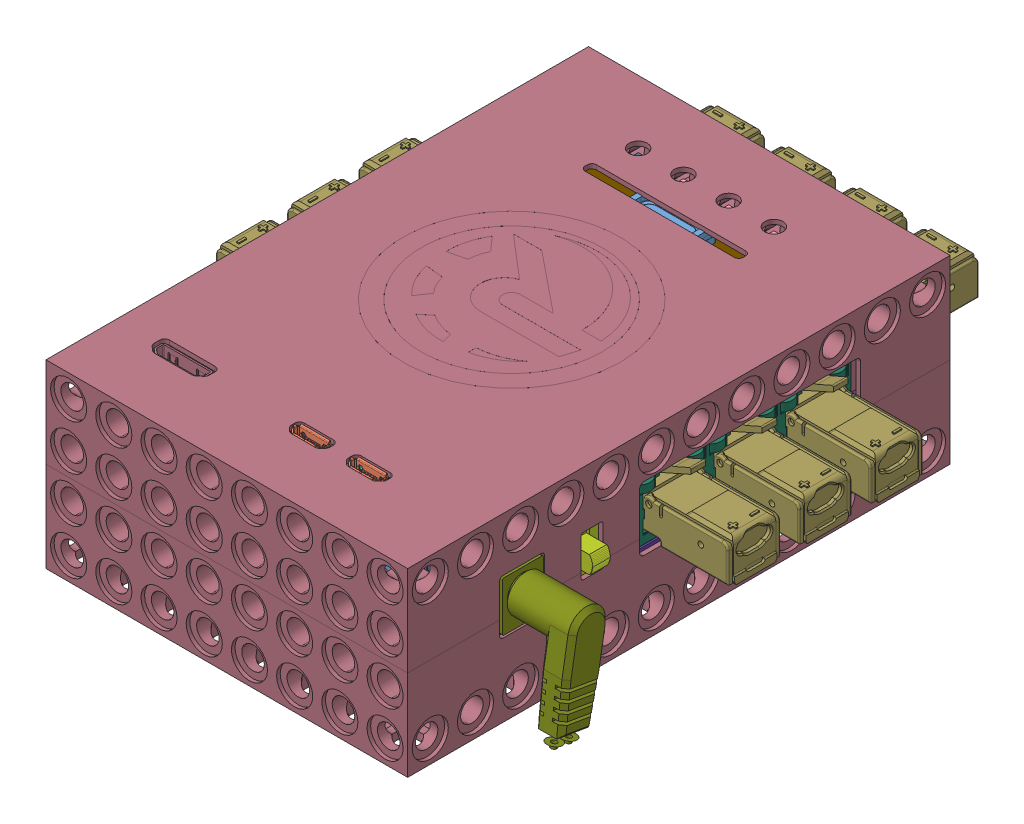
SolidWorks assembly PCBA_estimation_20190215, configuration Default. Lengths in mm. (continued)
Components (placement in the parent): (continued)
- RRRC_carrier_board-1: RRRC_carrier_board [Default] at (75.1836 8.28 47.3515) x (0 0 -1) z (0 1 0) size (102.74 81.4 21.81) (continued)
  - D1_CARRIER_3-1: D1_CARRIER_3 [Default] at origin size (1.05 0.65 0.44)
    - SOD-923_3-1: SOD-923_3 [Default] at (75.25 23.35 0) x (1 0 0) z (0 -1 0) size (1.05 0.44 0.65)
  - CON8_CARRIER_3-1: CON8_CARRIER_3 [Default] at origin size (17.2 66.95 18.85)
    - M-RJHSE-X38X-04-REVG1_3-1: M-RJHSE-X38X-04-REVG1_3 [Default] at (102.2431 7.1312 0.09) x (0 1 0) z (1 0 0) size (66.95 18.85 17.2)
  - CON7_CARRIER_3-1: CON7_CARRIER_3 [Default] at origin size (12.84 51.3 8.23)
    - Sullins_PPTC202LJBN-RC_3-1: Sullins_PPTC202LJBN-RC_3 [Default] at (8.4599 17.8499 -1.61) x (0 1 0) z (0 0 1) size (51.3 12.84 8.23)
  - CON6_CARRIER_3-1: CON6_CARRIER_3 [Default] at origin size (6.35 2.14 6.3)
    - SULLINS_GRPB051VWVN-RC_3-1: SULLINS_GRPB051VWVN-RC_3 [Default] at (-23.9866 70.2239 0) x (-1 0 0) z (0 1 0) size (6.35 6.3 2.14)
  - CON5_CARRIER_3-1: CON5_CARRIER_3 [Default] at origin size (3.02 8.01 9.01)
    - Molex_1051330001_3-1: Molex_1051330001_3 [Default] at (15.95 31.8001 2.7) x (0 1 0) z (0 0 -1) size (8.01 3.02 9.01)
  - CON4_CARRIER_3-1: CON4_CARRIER_3 [Default] at origin size (9 14.5 14.5)
    - CUI_INC_PJ-037A_3-1: CUI_INC_PJ-037A_3 [Default] at (9.6999 -1.4998 0) x (1 0 0) z (0 -1 0) size (9 14.5 14.5)
  - CON3_CARRIER_3-1: CON3_CARRIER_3 [Default] at origin size (51.17 16.61 18.92)
    - FCI_RJHSE538103-REVT1_3-1: FCI_RJHSE538103-REVT1_3 [Default] at (44.3006 76.8304 0.65) x (-1 0 0) z (0 1 0) size (51.17 18.92 16.61)
  - C58_CARRIER_3-1: C58_CARRIER_3 [Default] at origin size (1 0.5 0.5)
    - C_0402_3-1: C_0402_3 [Default] at (69.9 48.5 0) x (-1 0 0) z (0 0 1) size (1 0.5 0.5)
  - C38_CARRIER_3-1: C38_CARRIER_3 [Default] at origin size (0.5 1 0.5)
    - C_0402_3-1: C_0402_3 [Default] at (75.175 29.6 0) x (0 1 0) z (0 0 1) size (1 0.5 0.5)
  - C116_CARRIER_3-1: C116_CARRIER_3 [Default] at origin size (1 0.5 0.5)
    - C_0402_3-1: C_0402_3 [Default] at (71.9 53 0) x (1 0 0) z (0 0 1) size (1 0.5 0.5)
  - C115_CARRIER_3-1: C115_CARRIER_3 [Default] at origin size (1 0.5 0.5)
    - C_0402_3-1: C_0402_3 [Default] at (69.9 53 0) x (-1 0 0) z (0 0 1) size (1 0.5 0.5)
  - C114_CARRIER_3-1: C114_CARRIER_3 [Default] at origin size (0.5 1 0.5)
    - C_0402_3-1: C_0402_3 [Default] at (93.75 3 0) x (0 1 0) z (0 0 1) size (1 0.5 0.5)
  - C113_CARRIER_3-1: C113_CARRIER_3 [Default] at origin size (1 0.5 0.5)
    - C_0402_3-1: C_0402_3 [Default] at (71.95 39.35 0) x (1 0 0) z (0 0 1) size (1 0.5 0.5)
  - C109_CARRIER_3-1: C109_CARRIER_3 [Default] at origin size (1 0.5 0.5)
    - C_0402_3-1: C_0402_3 [Default] at (69.95 39.35 0) x (-1 0 0) z (0 0 1) size (1 0.5 0.5)
  - C108_CARRIER_3-1: C108_CARRIER_3 [Default] at origin size (1 0.5 0.5)
    - C_0402_3-1: C_0402_3 [Default] at (77.85 19.25 0) x (-1 0 0) z (0 0 1) size (1 0.5 0.5)
  - C107_CARRIER_3-1: C107_CARRIER_3 [Default] at origin size (1.6 3.2 1.6)
    - C_1206_3-1: C_1206_3 [Default] at (78.15 23.9 0) x (0 -1 0) z (0 0 1) size (3.2 1.6 1.6)
  - C106_CARRIER_3-1: C106_CARRIER_3 [Default] at origin size (3.2 1.6 1.6)
    - C_1206_3-1: C_1206_3 [Default] at (78.95 27.6 0) x (1 0 0) z (0 0 1) size (3.2 1.6 1.6)
  - C104_CARRIER_3-1: C104_CARRIER_3 [Default] at origin size (1 0.5 0.5)
    - C_0402_3-1: C_0402_3 [Default] at (71.9 43.825 0) x (1 0 0) z (0 0 1) size (1 0.5 0.5)
  - C98_CARRIER_3-1: C98_CARRIER_3 [Default] at origin size (1 0.5 0.5)
    - C_0402_3-1: C_0402_3 [Default] at (69.9 43.825 0) x (-1 0 0) z (0 0 1) size (1 0.5 0.5)
  - C97_CARRIER_3-1: C97_CARRIER_3 [Default] at origin size (1.6 3.2 1.6)
    - C_1206_3-1: C_1206_3 [Default] at (30.9 62.1 0) x (0 -1 0) z (0 0 1) size (3.2 1.6 1.6)
  - C96_CARRIER_3-1: C96_CARRIER_3 [Default] at origin size (1 0.5 0.5)
    - C_0402_3-1: C_0402_3 [Default] at (71.9 48.5 0) x (1 0 0) z (0 0 1) size (1 0.5 0.5)
  - C95_CARRIER_3-1: C95_CARRIER_3 [Default] at origin size (1 0.5 0.5)
    - C_0402_3-1: C_0402_3 [Default] at (16.6 19.725 0) x (1 0 0) z (0 0 1) size (1 0.5 0.5)
  - C94_CARRIER_3-1: C94_CARRIER_3 [Default] at origin size (1.6 3.2 1.6)
    - C_1206_3-1: C_1206_3 [Default] at (32.75 12.9 0) x (0 1 0) z (0 0 1) size (3.2 1.6 1.6)
  - C93_CARRIER_3-1: C93_CARRIER_3 [Default] at origin size (1.6 3.2 1.6)
    - C_1206_3-1: C_1206_3 [Default] at (17.05 12.9 0) x (0 1 0) z (0 0 1) size (3.2 1.6 1.6)
  - C92_CARRIER_3-1: C92_CARRIER_3 [Default] at origin size (1.6 3.2 1.6)
    - C_1206_3-1: C_1206_3 [Default] at (3.4 10.65 0) x (0 1 0) z (0 0 1) size (3.2 1.6 1.6)
  - C91_CARRIER_3-1: C91_CARRIER_3 [Default] at origin size (0.5 1 0.5)
    - C_0402_3-1: C_0402_3 [Default] at (88.95 74.5 0) x (0 -1 0) z (0 0 1) size (1 0.5 0.5)
  - C89_CARRIER_3-1: C89_CARRIER_3 [Default] at origin size (1.6 3.2 1.6)
    - C_1206_3-1: C_1206_3 [Default] at (20.075 27.05 0) x (0 -1 0) z (0 0 1) size (3.2 1.6 1.6)
  - C88_CARRIER_3-1: C88_CARRIER_3 [Default] at origin size (1 0.5 0.5)
    - C_0402_3-1: C_0402_3 [Default] at (66.9 56.6 0) x (1 0 0) z (0 0 1) size (1 0.5 0.5)
  - C87_CARRIER_3-1: C87_CARRIER_3 [Default] at origin size (1 0.5 0.5)
    - C_0402_3-1: C_0402_3 [Default] at (62.45 57.7 0) x (-1 0 0) z (0 0 1) size (1 0.5 0.5)
  - C85_CARRIER_3-1: C85_CARRIER_3 [Default] at origin size (1.2 2 1.2)
    - C_0805_3-1: C_0805_3 [Default] at (64.45 51.95 0.1) x (0 -1 0) z (0 0 1) size (2 1.2 1.2)
  - C83_CARRIER_3-1: C83_CARRIER_3 [Default] at origin size (1 0.5 0.5)
    - C_0402_3-1: C_0402_3 [Default] at (69.25 55.05 0) x (1 0 0) z (0 0 1) size (1 0.5 0.5)
  - C80_CARRIER_3-1: C80_CARRIER_3 [Default] at origin size (0.5 1 0.5)
    - C_0402_3-1: C_0402_3 [Default] at (79.875 22.925 0) x (0 -1 0) z (0 0 1) size (1 0.5 0.5)
  - C78_CARRIER_3-1: C78_CARRIER_3 [Default] at origin size (0.5 1 0.5)
    - C_0402_3-1: C_0402_3 [Default] at (79.85 25.425 0) x (0 1 0) z (0 0 1) size (1 0.5 0.5)
  - C69_CARRIER_3-1: C69_CARRIER_3 [Default] at origin size (1 0.5 0.5)
    - C_0402_3-1: C_0402_3 [Default] at (32.75 28.7 0) x (-1 0 0) z (0 0 1) size (1 0.5 0.5)
  - C68_CARRIER_3-1: C68_CARRIER_3 [Default] at origin size (1 0.5 0.5)
    - C_0402_3-1: C_0402_3 [Default] at (32.75 32.5 0) x (-1 0 0) z (0 0 1) size (1 0.5 0.5)
  - C67_CARRIER_3-1: C67_CARRIER_3 [Default] at origin size (0.5 1 0.5)
    - C_0402_3-1: C_0402_3 [Default] at (18.4 26.25 0) x (0 1 0) z (0 0 1) size (1 0.5 0.5)
  - C66_CARRIER_3-1: C66_CARRIER_3 [Default] at origin size (0.5 1 0.5)
    - C_0402_3-1: C_0402_3 [Default] at (19.475 30.6 0) x (0 1 0) z (0 0 1) size (1 0.5 0.5)
  - C65_CARRIER_3-1: C65_CARRIER_3 [Default] at origin size (1.6 3.2 1.6)
    - C_1206_3-1: C_1206_3 [Default] at (7.15 22.3 0) x (0 -1 0) z (0 0 1) size (3.2 1.6 1.6)
  - C64_CARRIER_3-1: C64_CARRIER_3 [Default] at origin size (0.5 1 0.5)
    - C_0402_3-1: C_0402_3 [Default] at (22.5 30.6 0) x (0 1 0) z (0 0 1) size (1 0.5 0.5)
  - C62_CARRIER_3-1: C62_CARRIER_3 [Default] at origin size (1 0.5 0.5)
    - C_0402_3-1: C_0402_3 [Default] at (33.025 62.8 0) x (-1 0 0) z (0 0 1) size (1 0.5 0.5)
  - C61_CARRIER_3-1: C61_CARRIER_3 [Default] at origin size (0.5 1 0.5)
    - C_0402_3-1: C_0402_3 [Default] at (7.325 64.75 0) x (0 -1 0) z (0 0 1) size (1 0.5 0.5)
  - C60_CARRIER_3-1: C60_CARRIER_3 [Default] at origin size (0.5 1 0.5)
    - C_0402_3-1: C_0402_3 [Default] at (7.325 66.75 0) x (0 1 0) z (0 0 1) size (1 0.5 0.5)
  - C59_CARRIER_3-1: C59_CARRIER_3 [Default] at origin size (2 1.2 1.2)
    - C_0805_3-1: C_0805_3 [Default] at (4.25 36.05 0.1) x (1 0 0) z (0 0 1) size (2 1.2 1.2)
  - C57_CARRIER_3-1: C57_CARRIER_3 [Default] at origin size (0.5 1 0.5)
    - C_0402_3-1: C_0402_3 [Default] at (14.95 21.275 0) x (0 -1 0) z (0 0 1) size (1 0.5 0.5)
  - C56_CARRIER_3-1: C56_CARRIER_3 [Default] at origin size (0.81 1.6 0.81)
    - C_0603_3-1: C_0603_3 [Default] at (6.5 30 0) x (0 -1 0) z (0 0 1) size (1.6 0.81 0.81)
  - C55_CARRIER_3-1: C55_CARRIER_3 [Default] at origin size (0.5 1 0.5)
    - C_0402_3-1: C_0402_3 [Default] at (1.2 51.75 0) x (0 1 0) z (0 0 1) size (1 0.5 0.5)
  - C54_CARRIER_3-1: C54_CARRIER_3 [Default] at origin size (1.6 3.2 1.6)
    - C_1206_3-1: C_1206_3 [Default] at (62.45 52.5 0) x (0 -1 0) z (0 0 1) size (3.2 1.6 1.6)
  - C52_CARRIER_3-1: C52_CARRIER_3 [Default] at origin size (1.6 3.2 1.6)
    - C_1206_3-1: C_1206_3 [Default] at (50.3 52.15 0) x (0 1 0) z (0 0 1) size (3.2 1.6 1.6)
  - C50_CARRIER_3-1: C50_CARRIER_3 [Default] at origin size (1.6 3.2 1.6)
    - C_1206_3-1: C_1206_3 [Default] at (42.1 51.85 0) x (0 1 0) z (0 0 1) size (3.2 1.6 1.6)
  - C48_CARRIER_3-1: C48_CARRIER_3 [Default] at origin size (1.6 3.2 1.6)
    - C_1206_3-1: C_1206_3 [Default] at (37.375 25.625 0) x (0 1 0) z (0 0 1) size (3.2 1.6 1.6)
  - C47_CARRIER_3-1: C47_CARRIER_3 [Default] at origin size (3.2 1.6 1.6)
    - C_1206_3-1: C_1206_3 [Default] at (34.325 18.15 0) x (-1 0 0) z (0 0 1) size (3.2 1.6 1.6)
  - C44_CARRIER_3-1: C44_CARRIER_3 [Default] at origin size (2 1.2 1.2)
    - C_0805_3-1: C_0805_3 [Default] at (3.9 60.9 0.1) x (1 0 0) z (0 0 1) size (2 1.2 1.2)
  - C43_CARRIER_3-1: C43_CARRIER_3 [Default] at origin size (0.81 1.6 0.81)
    - C_0603_3-1: C_0603_3 [Default] at (6.525 54.375 0) x (0 1 0) z (0 0 1) size (1.6 0.81 0.81)
  - C40_CARRIER_3-1: C40_CARRIER_3 [Default] at origin size (0.5 1 0.5)
    - C_0402_3-1: C_0402_3 [Default] at (5.05 23.25 0) x (0 1 0) z (0 0 1) size (1 0.5 0.5)
  - C45_CARRIER_3-1: C45_CARRIER_3 [Default] at origin size (0.5 1 0.5)
    - C_0402_3-1: C_0402_3 [Default] at (47.15 29.6 0) x (0 1 0) z (0 0 1) size (1 0.5 0.5)
  - C41_CARRIER_3-1: C41_CARRIER_3 [Default] at origin size (0.5 1 0.5)
    - C_0402_3-1: C_0402_3 [Default] at (60.15 29.6 0) x (0 1 0) z (0 0 1) size (1 0.5 0.5)
  - C26_CARRIER_3-1: C26_CARRIER_3 [Default] at origin size (3.2 1.6 1.6)
    - C_1206_3-1: C_1206_3 [Default] at (61.15 37.95 0) x (1 0 0) z (0 0 1) size (3.2 1.6 1.6)
  - C22_CARRIER_3-1: C22_CARRIER_3 [Default] at origin size (1.6 3.2 1.6)
    - C_1206_3-1: C_1206_3 [Default] at (70.725 33.025 0) x (0 1 0) z (0 0 1) size (3.2 1.6 1.6)
  - C20_CARRIER_3-1: C20_CARRIER_3 [Default] at origin size (1 0.5 0.5)
    - C_0402_3-1: C_0402_3 [Default] at (65.175 35.8 0) x (-1 0 0) z (0 0 1) size (1 0.5 0.5)
  - C18_CARRIER_3-1: C18_CARRIER_3 [Default] at origin size (0.5 1 0.5)
    - C_0402_3-1: C_0402_3 [Default] at (72.35 34.25 0) x (0 1 0) z (0 0 1) size (1 0.5 0.5)
  - C17_CARRIER_3-1: C17_CARRIER_3 [Default] at origin size (1 0.5 0.5)
    - C_0402_3-1: C_0402_3 [Default] at (69.325 19.575 0) x (-1 0 0) z (0 0 1) size (1 0.5 0.5)
  - C16_CARRIER_3-1: C16_CARRIER_3 [Default] at origin size (1 0.5 0.5)
    - C_0402_3-1: C_0402_3 [Default] at (73.375 19.575 0) x (-1 0 0) z (0 0 1) size (1 0.5 0.5)
  - C15_CARRIER_3-1: C15_CARRIER_3 [Default] at origin size (1 0.5 0.5)
    - C_0402_3-1: C_0402_3 [Default] at (70.85 22.55 0) x (1 0 0) z (0 0 1) size (1 0.5 0.5)
  - C14_CARRIER_3-1: C14_CARRIER_3 [Default] at origin size (2 1.2 1.2)
    - C_0805_3-1: C_0805_3 [Default] at (75.2 21.85 0.1) x (1 0 0) z (0 0 1) size (2 1.2 1.2)
  - C13_CARRIER_3-1: C13_CARRIER_3 [Default] at origin size (0.5 1 0.5)
    - C_0402_3-1: C_0402_3 [Default] at (15.55 44.05 0) x (0 -1 0) z (0 0 1) size (1 0.5 0.5)
  - C12_CARRIER_3-1: C12_CARRIER_3 [Default] at origin size (0.5 1 0.5)
    - C_0402_3-1: C_0402_3 [Default] at (15.35 48.85 0) x (0 -1 0) z (0 0 1) size (1 0.5 0.5)
  - C11_CARRIER_3-1: C11_CARRIER_3 [Default] at origin size (0.5 1 0.5)
    - C_0402_3-1: C_0402_3 [Default] at (35.3 54.025 0) x (0 1 0) z (0 0 1) size (1 0.5 0.5)
  - C10_CARRIER_3-1: C10_CARRIER_3 [Default] at origin size (1 0.5 0.5)
    - C_0402_3-1: C_0402_3 [Default] at (23.4 57.76 0) x (-1 0 0) z (0 0 1) size (1 0.5 0.5)
  - C9_CARRIER_3-1: C9_CARRIER_3 [Default] at origin size (1 0.5 0.5)
    - C_0402_3-1: C_0402_3 [Default] at (27 57.75 0) x (-1 0 0) z (0 0 1) size (1 0.5 0.5)
  - C8_CARRIER_3-1: C8_CARRIER_3 [Default] at origin size (1 0.5 0.5)
    - C_0402_3-1: C_0402_3 [Default] at (29.55 57.76 0) size (1 0.5 0.5)
  - C7_CARRIER_3-1: C7_CARRIER_3 [Default] at origin size (1 0.5 0.5)
    - C_0402_3-1: C_0402_3 [Default] at (22.1 38.15 0) x (1 0 0) z (0 0 1) size (1 0.5 0.5)
  - C6_CARRIER_3-1: C6_CARRIER_3 [Default] at origin size (1 0.5 0.5)
    - C_0402_3-1: C_0402_3 [Default] at (26.5 38.05 0) x (-1 0 0) z (0 0 1) size (1 0.5 0.5)
  - C5_CARRIER_3-1: C5_CARRIER_3 [Default] at origin size (1 0.5 0.5)
    - C_0402_3-1: C_0402_3 [Default] at (26.5 37.05 0) x (-1 0 0) z (0 0 1) size (1 0.5 0.5)
  - C4_CARRIER_3-1: C4_CARRIER_3 [Default] at origin size (0.5 1 0.5)
    - C_0402_3-1: C_0402_3 [Default] at (35.25 51.4 0) x (0 1 0) z (0 0 1) size (1 0.5 0.5)
  - C3_CARRIER_3-1: C3_CARRIER_3 [Default] at origin size (3.2 1.6 1.6)
    - C_1206_3-1: C_1206_3 [Default] at (38.3 51.75 0) x (-1 0 0) z (0 0 1) size (3.2 1.6 1.6)
  - C2_CARRIER_3-1: C2_CARRIER_3 [Default] at origin size (1.6 3.2 1.6)
    - C_1206_3-1: C_1206_3 [Default] at (33.15 59.775 0) x (0 -1 0) z (0 0 1) size (3.2 1.6 1.6)
  - C1_CARRIER_3-1: C1_CARRIER_3 [Default] at origin size (0.5 1 0.5)
    - C_0402_3-1: C_0402_3 [Default] at (22.95 35.55 0) x (0 1 0) z (0 0 1) size (1 0.5 0.5)
- RRRC_LED_board-1: RRRC_LED_board [Default] at (7.6864 26.7896 -45.8485) x (0 0 1) z (0 1 0) size (80 58 5.61)
  - Board_LEDs-1: Board_LEDs [Default] at origin size (80 58 1.6)
    - Open CASCADE STEP translator 6.8 1.1.1_3-1: Open CASCADE STEP translator 6.8 1.1.1_3 [Default] at (0 0 -1.6) size (80 58 1.6)
  - LS2_LEDs-1: LS2_LEDs [Default] at origin size (11 15 4.4)
    - AS01508AO-SC-R-1: AS01508AO-SC-R [Default] at (9.1999 22.6001 2.05) x (0 1 0) z (0 0 -1) size (15 11 4.4)
  - R2_LEDs-1: R2_LEDs [Default] at origin size (0.55 1.15 0.41)
    - R_0402_4-1: R_0402_4 [Default] at (15.225 50.25 0) x (0 -1 0) z (-1 0 0) size (1.15 0.41 0.55)
  - R1_LEDs-1: R1_LEDs [Default] at origin size (0.55 1.15 0.41)
    - R_0402_4-1: R_0402_4 [Default] at (9.325 49.825 0) x (0 -1 0) z (-1 0 0) size (1.15 0.41 0.55)
  - Q1_LEDs-1: Q1_LEDs [Default] at origin size (3 3.05 1.41)
    - SOT95P255X140-3N_4-1: SOT95P255X140-3N_4 [Default] at (12.15 50.275 0) x (-1 0 0) z (0 0 1) size (3 3.05 1.41)
  - LED16_LEDs-1: LED16_LEDs [Default] at origin size (5 5 1.6)
    - 6300770016-1: 6300770016 [Default] at (46 7 0) size (5 5 1.6)
      - Extruded_4-1: Extruded_4 [Default] at origin size (5 5 1.6)
  - LED15_LEDs-1: LED15_LEDs [Default] at origin size (6.83 6.83 1.6)
    - 6300767936-1: 6300767936 [Default] at (57 9.9474 0) size (6.83 6.83 1.6)
      - Extruded_4_2-1: Extruded_4_2 [Default] at origin size (6.83 6.83 1.6)
  - LED14_LEDs-1: LED14_LEDs [Default] at origin size (6.83 6.83 1.6)
    - 6300767056-1: 6300767056 [Default] at (65.0526 18 0) size (6.83 6.83 1.6)
      - Extruded_4_3-1: Extruded_4_3 [Default] at origin size (6.83 6.83 1.6)
  - LED13_LEDs-1: LED13_LEDs [Default] at origin size (5 5 1.6)
    - 6300770016-1-1: 6300770016-1 [Default] at (68 29 0) size (5 5 1.6)
      - Extruded_4-1: Extruded_4 [Default] at origin size (5 5 1.6)
  - LED12_LEDs-1: LED12_LEDs [Default] at origin size (6.83 6.83 1.6)
    - 6300767936-1-1: 6300767936-1 [Default] at (65.0526 40 0) size (6.83 6.83 1.6)
      - Extruded_4_2-1: Extruded_4_2 [Default] at origin size (6.83 6.83 1.6)
  - LED11_LEDs-1: LED11_LEDs [Default] at origin size (6.83 6.83 1.6)
    - 6300767056-1-1: 6300767056-1 [Default] at (57 48.0526 0) size (6.83 6.83 1.6)
      - Extruded_4_3-1: Extruded_4_3 [Default] at origin size (6.83 6.83 1.6)
  - LED10_LEDs-1: LED10_LEDs [Default] at origin size (5 5 1.6)
    - 6300770016-2-1: 6300770016-2 [Default] at (46 51 0) size (5 5 1.6)
      - Extruded_4-1: Extruded_4 [Default] at origin size (5 5 1.6)
  - LED9_LEDs-1: LED9_LEDs [Default] at origin size (6.83 6.83 1.6)
    - 6300765456-1: 6300765456 [Default] at (35 48.0526 0) size (6.83 6.83 1.6)
      - Extruded_4_4-1: Extruded_4_4 [Default] at origin size (6.83 6.83 1.6)
  - LED8_LEDs-1: LED8_LEDs [Default] at origin size (6.83 6.83 1.6)
    - 6300764256-1: 6300764256 [Default] at (26.9474 40 0) size (6.83 6.83 1.6)
      - Extruded_4_5-1: Extruded_4_5 [Default] at origin size (6.83 6.83 1.6)
  - LED7_LEDs-1: LED7_LEDs [Default] at origin size (5 5 1.6)
    - 6300770016-3-1: 6300770016-3 [Default] at (24 29 0) size (5 5 1.6)
      - Extruded_4-1: Extruded_4 [Default] at origin size (5 5 1.6)
  - LED6_LEDs-1: LED6_LEDs [Default] at origin size (6.83 6.83 1.6)
    - 6300767936-2-1: 6300767936-2 [Default] at (26.9474 18 0) size (6.83 6.83 1.6)
      - Extruded_4_2-1: Extruded_4_2 [Default] at origin size (6.83 6.83 1.6)
  - LED5_LEDs-1: LED5_LEDs [Default] at origin size (6.83 6.83 1.6)
    - 6300766096-1: 6300766096 [Default] at (35 9.95 0) size (6.83 6.83 1.6)
      - Extruded_4_6-1: Extruded_4_6 [Default] at origin size (6.83 6.83 1.6)
  - LED4_LEDs-1: LED4_LEDs [Default] at origin size (5 5 1.6)
    - 6300768656-1: 6300768656 [Default] at (3 14 0) size (5 5 1.6)
      - Extruded_4_7-1: Extruded_4_7 [Default] at origin size (5 5 1.6)
  - LED3_LEDs-1: LED3_LEDs [Default] at origin size (5 5 1.6)
    - 6300770016-4-1: 6300770016-4 [Default] at (3 24 0) size (5 5 1.6)
      - Extruded_4-1: Extruded_4 [Default] at origin size (5 5 1.6)
  - LED2_LEDs-1: LED2_LEDs [Default] at origin size (5 5 1.6)
    - 6300770016-5-1: 6300770016-5 [Default] at (3 34 0) size (5 5 1.6)
      - Extruded_4-1: Extruded_4 [Default] at origin size (5 5 1.6)
  - LED1_LEDs-1: LED1_LEDs [Default] at origin size (5 5 1.6)
    - 6300770016-6-1: 6300770016-6 [Default] at (3 44 0) size (5 5 1.6)
      - Extruded_4-1: Extruded_4 [Default] at origin size (5 5 1.6)
  - C16_LEDs-1: C16_LEDs [Default] at origin size (1 0.5 0.5)
    - C_0402_4-1: C_0402_4 [Default] at (46 11.38 0) x (-1 0 0) z (0 0 1) size (1 0.5 0.5)
  - C15_LEDs-1: C15_LEDs [Default] at origin size (1.12 0.93 0.5)
    - C_0402_4-1: C_0402_4 [Default] at (54.81 13.7406 0) x (-0.866025 -0.5 0) z (0 0 1) size (1 0.5 0.5)
  - C14_LEDs-1: C14_LEDs [Default] at origin size (0.93 1.12 0.5)
    - C_0402_4-1: C_0402_4 [Default] at (61.2594 20.19 0) x (-0.5 -0.866025 0) z (0 0 1) size (1 0.5 0.5)
  - C13_LEDs-1: C13_LEDs [Default] at origin size (0.5 1 0.5)
    - C_0402_4-1: C_0402_4 [Default] at (63.62 29 0) x (0 -1 0) z (0 0 1) size (1 0.5 0.5)
  - C12_LEDs-1: C12_LEDs [Default] at origin size (0.93 1.12 0.5)
    - C_0402_4-1: C_0402_4 [Default] at (61.2594 37.81 0) x (0.5 -0.866025 0) z (0 0 1) size (1 0.5 0.5)
  - C11_LEDs-1: C11_LEDs [Default] at origin size (1.12 0.93 0.5)
    - C_0402_4-1: C_0402_4 [Default] at (54.81 44.2594 0) x (0.866025 -0.5 0) z (0 0 1) size (1 0.5 0.5)
  - C10_LEDs-1: C10_LEDs [Default] at origin size (1 0.5 0.5)
    - C_0402_4-1: C_0402_4 [Default] at (46 46.62 0) x (1 0 0) z (0 0 1) size (1 0.5 0.5)
  - C9_LEDs-1: C9_LEDs [Default] at origin size (1.12 0.93 0.5)
    - C_0402_4-1: C_0402_4 [Default] at (37.19 44.2594 0) x (0.866025 0.5 0) z (0 0 1) size (1 0.5 0.5)
  - C8_LEDs-1: C8_LEDs [Default] at origin size (0.93 1.12 0.5)
    - C_0402_4-1: C_0402_4 [Default] at (30.7406 37.81 0) x (0.5 0.866025 0) z (0 0 1) size (1 0.5 0.5)
  - C7_LEDs-1: C7_LEDs [Default] at origin size (0.5 1 0.5)
    - C_0402_4-1: C_0402_4 [Default] at (28.38 29 0) x (0 1 0) z (0 0 1) size (1 0.5 0.5)
  - C6_LEDs-1: C6_LEDs [Default] at origin size (0.93 1.12 0.5)
    - C_0402_4-1: C_0402_4 [Default] at (30.7406 20.19 0) x (-0.5 0.866025 0) z (0 0 1) size (1 0.5 0.5)
  - C5_LEDs-1: C5_LEDs [Default] at origin size (1.12 0.93 0.5)
    - C_0402_4-1: C_0402_4 [Default] at (37.19 13.7406 0) x (-0.866025 0.5 0) z (0 0 1) size (1 0.5 0.5)
  - C4_LEDs-1: C4_LEDs [Default] at origin size (1 0.5 0.5)
    - C_0402_4-1: C_0402_4 [Default] at (4.075 48.375 0) x (1 0 0) z (0 0 1) size (1 0.5 0.5)
  - C3_LEDs-1: C3_LEDs [Default] at origin size (1 0.5 0.5)
    - C_0402_4-1: C_0402_4 [Default] at (4.075 38.25 0) x (1 0 0) z (0 0 1) size (1 0.5 0.5)
  - C2_LEDs-1: C2_LEDs [Default] at origin size (1 0.5 0.5)
    - C_0402_4-1: C_0402_4 [Default] at (4.075 28.3 0) x (1 0 0) z (0 0 1) size (1 0.5 0.5)
  - C1_LEDs-1: C1_LEDs [Default] at origin size (1 0.5 0.5)
    - C_0402_4-1: C_0402_4 [Default] at (4.075 18.3 0) x (1 0 0) z (0 0 1) size (1 0.5 0.5)
- 17x8669_2213145-2-1: 17x8669_2213145-2 [Default] at (44.4306 13.6886 -45.3782) size (11.77 14.58 29.91)
- 17x8669_2213145-2-2: 17x8669_2213145-2 [Default] at (60.1786 13.6886 -45.3782) size (11.77 14.58 29.91)
- 17x8669_2213145-2-3: 17x8669_2213145-2 [Default] at (8.4158 13.6886 -12.7277) x (0 0 -1) z (1 0 0) size (11.77 14.58 29.91)
- 17x8669_2213145-2-4: 17x8669_2213145-2 [Default] at (12.9346 13.6886 -45.3782) size (11.77 14.58 29.91)
- 17x8669_2213145-2-5: 17x8669_2213145-2 [Default] at (8.4158 13.6886 3.0203) x (0 0 -1) z (1 0 0) size (11.77 14.58 29.91)
- 17x8669_2213145-2-6: 17x8669_2213145-2 [Default] at (64.9514 13.6886 3.2743) x (0 0 1) z (-1 0 0) size (11.77 14.58 29.91)
- 17x8669_2213145-2-7: 17x8669_2213145-2 [Default] at (64.9514 13.6886 -12.4737) x (0 0 1) z (-1 0 0) size (11.77 14.58 29.91)
- 17x8669_2213145-2-8: 17x8669_2213145-2 [Default] at (64.9514 13.6886 -28.2217) x (0 0 1) z (-1 0 0) size (11.77 14.58 29.91)
- 17x8669_2213145-2-9: 17x8669_2213145-2 [Default] at (8.4158 13.6886 -28.4757) x (0 0 -1) z (1 0 0) size (11.77 14.58 29.91)
- 17x8669_2213145-2-10: 17x8669_2213145-2 [Default] at (28.6826 13.6886 -45.3782) size (11.77 14.58 29.91)
- BRcA-1: BRcA [Default] at (36.6864 -8.3104 3.1515) x (0 0 -1) z (1 0 0) size (120 40 80)
- Micro SD Card-1: Micro SD Card [Default] at (-3.3136 19.4788 48.6272) x (0 -1 0) z (-1 0 0) size (11.21 1.12 15.03)
- JHY_813270_2000mAh-1: JHY_813270_2000mAh [Default] at (37.0596 17.0896 16.1186) x (1 0 0) z (0 1 0) size (32 70.5 8.1)
- Power_Jack_2mm-1: Power_Jack_2mm [Default] at (91.9336 14.78 37.8515) x (0 0.985977 -0.166882) z (0 0.166882 0.985977) size (26 26.35 8.3)
- PR(E,P)C020DAAN-RC-1: PR(E,P)C020DAAN-RC [Default] at (7.5875 4.1126 49.4916) x (1 0 0) z (0 1 0) size (50.8 11.37 5.08)
- SHR-05V-S-B-1: SHR-05V-S-B [Default] at (41.6836 13.455 8.5516) x (0 0 1) z (0 -1 0) size (8 2.8 5)
